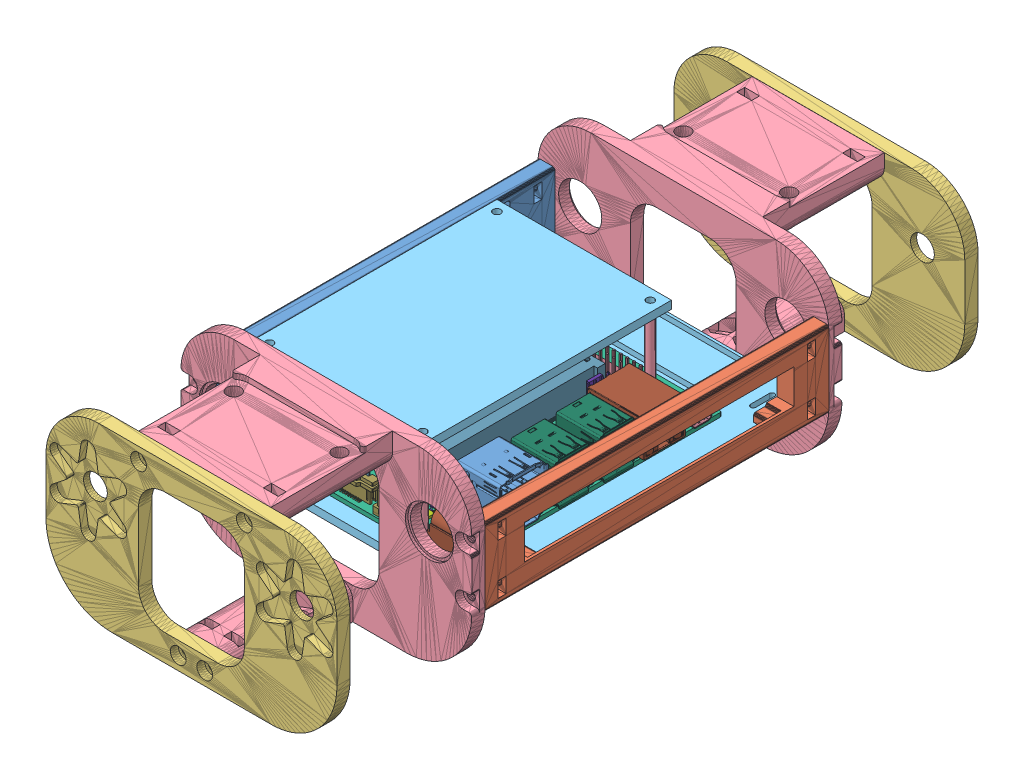
SolidWorks assembly torsol_with_jestson, configuration Default. Lengths in mm. (continued)
Components (placement in the parent): (continued)
- plate_with_jetson-1: plate_with_jetson [Default] at (-139.2728 38.0458 18.6623) x (-1 0 0) z (0 -1 0) size (107 134 44.9) (continued)
  - Jetson nano_fixed.step-1: Jetson nano_fixed.step [Default] at (-69.1681 -61.3023 -1.45) x (0 1 0) z (0 0 -1) size (100 81.03 30.51) (continued)
    - 142-13449-1000-A02_ASM.step-1: 142-13449-1000-A02_ASM.step [Default] at origin size (100 81.03 23.19) (continued)
      - 074-0102-000_4.step-1: 074-0102-000_4.step [Default] at (0.254 44.36 1.575) x (0 1 0) z (0 0 1) size (10.16 5.08 11.6)
      - 064-0400-000_1.step-1: 064-0400-000_1.step [Default] at (73.75 7.77 1.575) size (10.16 5.8 13.5)
      - MEC_STANDOFF_PTH_620C380P.step-1: MEC_STANDOFF_PTH_620C380P.step [Default] at (40.276 40.3 1.575) x (0 1 0) z (0 0 1) size (6.2 6.2 0.73)
      - 090-0231-000_1.step-1: 090-0231-000_1.step [Default] at (35.3 0.7 1.575) x (-1 0 0) z (0 0 1) size (2.5 1.55 0.55)
      - 090-0231-000_1.step-2: 090-0231-000_1.step [Default] at (52.25 0.7 1.575) x (-1 0 0) z (0 0 1) size (2.5 1.55 0.55)
      - 090-0231-000_1.step-3: 090-0231-000_1.step [Default] at (56.05 0.7 1.575) size (2.5 1.55 0.55)
      - 090-0231-000_1.step-4: 090-0231-000_1.step [Default] at (59.65 0.7 1.575) size (2.5 1.55 0.55)
      - 090-0231-000_1.step-5: 090-0231-000_1.step [Default] at (39.1 0.7 1.575) size (2.5 1.55 0.55)
      - 090-0231-000_1.step-6: 090-0231-000_1.step [Default] at (43.1 0.7 1.575) size (2.5 1.55 0.55)
      - 090-0231-000_1.step-7: 090-0231-000_1.step [Default] at (14.6 1.8 1.575) size (2.5 1.55 0.55)
      - 090-0231-000_1.step-8: 090-0231-000_1.step [Default] at (19.1 1.8 1.575) size (2.5 1.55 0.55)
      - 090-0231-000_1.step-9: 090-0231-000_1.step [Default] at (22.5 1.4 1.575) size (2.5 1.55 0.55)
      - 090-0231-000_1.step-10: 090-0231-000_1.step [Default] at (28.45 3.35 1.575) size (2.5 1.55 0.55)
      - 090-0231-000_1.step-11: 090-0231-000_1.step [Default] at (31.65 3.35 1.575) size (2.5 1.55 0.55)
      - 074-0223-000_2.step-1: 074-0223-000_2.step [Default] at (5.85 53.25 1.575) x (0 1 0) z (0 0 1) size (15.24 2.54 11.6)
      - 131-0832-000_2.step-1: 131-0832-000_2.step [Default] at (56.3 54.7 1.575) x (0 -1 0) z (0 0 1) size (4.96 4.06 1.8)
      - 115-0836-000_1.step-1: 115-0836-000_1.step [Default] at (21.1 56.6 1.575) size (2.9 3.58 1.45)
      - 115-0836-000_1.step-2: 115-0836-000_1.step [Default] at (11.8 42.3 1.575) size (2.9 3.58 1.45)
      - 315-0620-000_1.step-1: 315-0620-000_1.step [Default] at (72.1 53.4 1.575) x (0 -1 0) z (0 0 1) size (2.9 3.58 1.1)
      - 315-1062-000_1.step-1: 315-1062-000_1.step [Default] at (26.8 25.15 1.575) x (0 -1 0) z (0 0 1) size (2.9 3.58 1.45)
      - 170-0285-000_1.step-1: 170-0285-000_1.step [Default] at (28.72 57.28 1.575) x (0 1 0) z (0 0 1) size (4.9 7.21 1.75)
      - 115-0138-000_1.step-1: 115-0138-000_1.step [Default] at (9.15 48.55 1.575) x (0 1 0) z (0 0 1) size (2 2.88 1.1)
      - 115-1821-000_1.step-1: 115-1821-000_1.step [Default] at (3.3 40.8 1.575) x (-1 0 0) z (0 0 1) size (2 2.88 1.1)
      - 115-1821-000_1.step-2: 115-1821-000_1.step [Default] at (6.25 39.55 1.575) x (0 -1 0) z (0 0 1) size (2 2.88 1.1)
      - 115-0742-000_2.step-1: 115-0742-000_2.step [Default] at (3.05 46.85 1.575) size (2 2.88 1.1)
      - 115-0742-000_2.step-2: 115-0742-000_2.step [Default] at (3.05 51.65 1.575) x (-1 0 0) z (0 0 1) size (2 2.88 1.1)
      - 115-1821-000_1.step-3: 115-1821-000_1.step [Default] at (59.6 27.6 1.575) x (0 1 0) z (0 0 1) size (2 2.88 1.1)
      - 091-0022-000_1.step-1: 091-0022-000_1.step [Default] at (-0.95 5.7 1.575) size (2 2.51 1.1)
      - 091-0023-000_1.step-1: 091-0023-000_1.step [Default] at (15.25 29.9 1.575) x (0 -1 0) z (0 0 1) size (2 2.51 1.1)
      - 080-1368-000_1.step-1: 080-1368-000_1.step [Default] at (88 -14.3 1.575) size (10.99 7.28 4.95)
      - 080-1656-000_3.step-1: 080-1656-000_3.step [Default] at (44 16.6 1.575) x (-1 0 0) z (0 0 1) size (77.5 25.85 9.76)
      - 090-0243-000_1.step-1: 090-0243-000_1.step [Default] at (8.5 -4.1 1.575) x (-1 0 0) z (0 0 1) size (1.41 0.61 0.45)
      - 090-0243-000_1.step-2: 090-0243-000_1.step [Default] at (9.95 -3.7 1.575) x (0 1 0) z (0 0 1) size (1.41 0.61 0.45)
      - 090-0243-000_1.step-3: 090-0243-000_1.step [Default] at (9.5 -10.95 1.575) x (-1 0 0) z (0 0 1) size (1.41 0.61 0.45)
      - 090-0243-000_1.step-4: 090-0243-000_1.step [Default] at (9.8 -6.25 1.575) x (-1 0 0) z (0 0 1) size (1.41 0.61 0.45)
      - 090-0243-000_1.step-5: 090-0243-000_1.step [Default] at (9.5 -9.5 1.575) x (-1 0 0) z (0 0 1) size (1.41 0.61 0.45)
      - 090-0172-000_1.step-1: 090-0172-000_1.step [Default] at (90.6 -5 1.575) size (1.41 0.61 0.55)
      - 090-0172-000_1.step-2: 090-0172-000_1.step [Default] at (88.8 -5 1.575) x (-1 0 0) z (0 0 1) size (1.41 0.61 0.55)
      - 115-2177-000_2.step-1: 115-2177-000_2.step [Default] at (12.7 51.35 1.575) x (0 1 0) z (0 0 1) size (1.8 1.71 0.4)
      - 090-0233-000_1.step-1: 090-0233-000_1.step [Default] at (83.5 -6.6 1.575) size (3.3 1.3 0.74)
      - 064-0374-000_2.step-1: 064-0374-000_2.step [Default] at (19.75 -9.65 1.575) size (18.11 18.56 21.86)
      - 115-2628-000_3.step-1: 115-2628-000_3.step [Default] at (25.2 41.2 1.575) size (9.5 9.5 0.9)
      - 092-0073-000_1.step-1: 092-0073-000_1.step [Default] at (93.35 -4.75 1.575) x (-1 0 0) z (0 0 1) size (2.46 0.81 0.9)
      - IND_SMD_0402_H060.step-1: IND_SMD_0402_H060.step [Default] at (12.85 29.9 1.575) x (-1 0 0) z (0 0 1) size (1 0.5 0.6)
      - 1206_H190.step-1: 1206_H190.step [Default] at (82 18.8 1.575) x (0 1 0) z (0 0 1) size (3.2 1.6 1.9)
      - 1206_H190.step-2: 1206_H190.step [Default] at (81.95 13.5 1.575) x (0 -1 0) z (0 0 1) size (3.2 1.6 1.9)
      - 300-0868-000_3.step-1: 300-0868-000_3.step [Default] at (69.6 4 1.575) x (-1 0 0) z (0 0 1) size (1 0.6 0.4)
      - 300-0868-000_3.step-2: 300-0868-000_3.step [Default] at (9.55 0.95 1.575) size (1 0.6 0.4)
      - 300-0868-000_3.step-3: 300-0868-000_3.step [Default] at (19.6 31.45 1.575) x (0 -1 0) z (0 0 1) size (1 0.6 0.4)
      - 300-0868-000_3.step-4: 300-0868-000_3.step [Default] at (91.45 -2.45 1.575) x (-1 0 0) z (0 0 1) size (1 0.6 0.4)
      - 300-0868-000_3.step-5: 300-0868-000_3.step [Default] at (84.6 -5.1 1.575) size (1 0.6 0.4)
      - 300-0868-000_3.step-6: 300-0868-000_3.step [Default] at (66.725 5.875 1.575) x (0 -1 0) z (0 0 1) size (1 0.6 0.4)
      - 300-0868-000_3.step-7: 300-0868-000_3.step [Default] at (20.8 31.45 1.575) x (0 -1 0) z (0 0 1) size (1 0.6 0.4)
      - 300-0868-000_3.step-8: 300-0868-000_3.step [Default] at (62.9 31.35 1.575) x (-1 0 0) z (0 0 1) size (1 0.6 0.4)
      - 300-0868-000_3.step-9: 300-0868-000_3.step [Default] at (65.475 4.8 1.575) x (-1 0 0) z (0 0 1) size (1 0.6 0.4)
      - 300-0868-000_3.step-10: 300-0868-000_3.step [Default] at (63.9 33.85 1.575) x (-1 0 0) z (0 0 1) size (1 0.6 0.4)
      - 300-0868-000_3.step-11: 300-0868-000_3.step [Default] at (15.65 27.9 1.575) size (1 0.6 0.4)
      - 300-0868-000_3.step-12: 300-0868-000_3.step [Default] at (11.8 6.1 1.575) x (0 1 0) z (0 0 1) size (1 0.6 0.4)
      - 300-0868-000_3.step-13: 300-0868-000_3.step [Default] at (22.1 6.25 1.575) x (0 1 0) z (0 0 1) size (1 0.6 0.4)
      - 300-0869-000_3.step-1: 300-0869-000_3.step [Default] at (9.65 8.1 1.575) x (0 -1 0) z (0 0 1) size (1 0.6 0.53)
      - 300-0402-000_1.step-1: 300-0402-000_1.step [Default] at (20.8 26.45 1.575) x (0 -1 0) z (0 0 1) size (2 2.69 1.1)
      - 300-0560-000_1.step-1: 300-0560-000_1.step [Default] at (6.8 43.65 1.575) x (-1 0 0) z (0 0 1) size (2 2.69 1.1)
      - 174-0159-000_2.step-1: 174-0159-000_2.step [Default] at (61.49 57.15 1.575) x (-1 0 0) z (0 0 1) size (2 3.52 0.6)
      - 064-0373-000_2.step-1: 064-0373-000_2.step [Default] at (72.95 -7.825 1.575) size (17.8 21.61 17.46)
      - 064-0375-000_2.step-1: 064-0375-000_2.step [Default] at (19.751 -12.275 1.575) size (16.2 5.58 0.01)
      - 074-0221-000_3.step-1: 074-0221-000_3.step [Default] at (86 29 1.575) x (0 1 0) z (0 0 1) size (50.8 5.08 11.6)
      - 2016MM_H100.step-1: 2016MM_H100.step [Default] at (24.5 49.25 1.575) x (0 1 0) z (0 0 1) size (2 1.6 1)
      - 065-0656-000_2.step-1: 065-0656-000_2.step [Default] at (55.6 -10.04 1.575) x (-1 0 0) z (0 0 1) size (16.19 17.45 19.62)
      - 065-0656-000_2.step-2: 065-0656-000_2.step [Default] at (38.6 -10.04 1.575) x (-1 0 0) z (0 0 1) size (16.19 17.45 19.62)
      - 115-1921-000_3.step-1: 115-1921-000_3.step [Default] at (80.45 50.52 1.575) x (0 -1 0) z (0 0 1) size (5 4 1)
      - 115-1921-000_3.step-2: 115-1921-000_3.step [Default] at (80.4 34.5 1.575) x (0 -1 0) z (0 0 1) size (5 4 1)
      - 115-1921-000_3.step-3: 115-1921-000_3.step [Default] at (77.2 25.9 1.575) x (0 -1 0) z (0 0 1) size (5 4 1)
      - 085-0328-000_2.step-1: 085-0328-000_2.step [Default] at (16.28 36.32 1.575) x (0 -1 0) z (0 0 1) size (3.81 2.5 0.6)
      - 074-0216-000_2.step-1: 074-0216-000_2.step [Default] at (92.14 58 1.575) x (-1 0 0) z (0 0 1) size (4.83 5 11.5)
      - 060-0002-000_1.step-1: 060-0002-000_1.step [Default] at (41.2 57.9 1.575) x (0 -1 0) z (0 0 1) size (5.1 5.4 1.68)
      - 316-0697-000_1.step-1: 316-0697-000_1.step [Default] at (50.6 58.1 1.575) x (0 -1 0) z (0 0 1) size (3 3.72 0.8)
      - 032-0256-000_1.step-1: 032-0256-000_1.step [Default] at (5.925 9.425 1.575) size (4.22 2.82 2)
      - 041-0092-000_1.step-1: 041-0092-000_1.step [Default] at (46.9 54.9 1.575) x (0 -1 0) z (0 0 1) size (4.22 2.82 1.2)
      - 080-1243-000_3.step-1: 080-1243-000_3.step [Default] at (69.9 40.3 1.575) x (0 -1 0) z (0 0 1) size (21.9 9.1 4.8)
      - 102-0066-000_2.step-1: 102-0066-000_2.step [Default] at (18 4.2 1.575) size (1 1.86 0.61)
      - 102-0066-000_2.step-2: 102-0066-000_2.step [Default] at (13.55 4.2 1.575) size (1 1.86 0.61)
      - 102-0066-000_2.step-3: 102-0066-000_2.step [Default] at (32.45 5.81 1.575) size (1 1.86 0.61)
      - 102-0066-000_2.step-4: 102-0066-000_2.step [Default] at (27.65 5.81 1.575) size (1 1.86 0.61)
      - 102-0066-000_2.step-5: 102-0066-000_2.step [Default] at (20.15 4.2 1.575) size (1 1.86 0.61)
      - 102-0066-000_2.step-6: 102-0066-000_2.step [Default] at (15.75 4.2 1.575) size (1 1.86 0.61)
      - 102-0066-000_2.step-7: 102-0066-000_2.step [Default] at (29.25 5.81 1.575) size (1 1.86 0.61)
      - 102-0066-000_2.step-8: 102-0066-000_2.step [Default] at (30.85 5.81 1.575) size (1 1.86 0.61)
      - 102-0037-000_1.step-1: 102-0037-000_1.step [Default] at (55.2 2.95 1.575) x (-1 0 0) z (0 0 1) size (1 1.86 0.91)
      - 102-0037-000_1.step-2: 102-0037-000_1.step [Default] at (39.99 2.87 1.575) x (-1 0 0) z (0 0 1) size (1 1.86 0.91)
      - 102-0037-000_1.step-3: 102-0037-000_1.step [Default] at (60.55 2.95 1.575) x (-1 0 0) z (0 0 1) size (1 1.86 0.91)
      - 102-0037-000_1.step-4: 102-0037-000_1.step [Default] at (38.22 2.87 1.575) x (-1 0 0) z (0 0 1) size (1 1.86 0.91)
      - 0805_H140.step-1: 0805_H140.step [Default] at (8.1 -2.1 1.575) size (2.01 1.25 1.4)
      - 0805_H150.step-1: 0805_H150.step [Default] at (82.9 -8.4 1.575) x (-1 0 0) z (0 0 1) size (2.01 1.25 1.5)
      - 0603_H100.step-1: 0603_H100.step [Default] at (6.1 41.525 1.575) x (-1 0 0) z (0 0 1) size (1.6 0.81 1)
      - 0603_H060.step-1: 0603_H060.step [Default] at (63.25 -12 1.575) x (0 1 0) z (0 0 1) size (1.6 0.81 0.6)
      - 0603_H060.step-2: 0603_H060.step [Default] at (63.8 -0.7 1.575) x (0 -1 0) z (0 0 1) size (1.6 0.81 0.6)
      - 0603_H060.step-3: 0603_H060.step [Default] at (82.4 -10 1.575) x (-1 0 0) z (0 0 1) size (1.6 0.81 0.6)
      - 0603_H100.step-2: 0603_H100.step [Default] at (9.486 -7.5 1.575) x (-1 0 0) z (0 0 1) size (1.6 0.81 1)
      - 0603_H100.step-3: 0603_H100.step [Default] at (17.4 57.4 1.575) x (0 -1 0) z (0 0 1) size (1.6 0.81 1)
      - 0603_H100.step-4: 0603_H100.step [Default] at (30.35 25.9 1.575) x (0 -1 0) z (0 0 1) size (1.6 0.81 1)
      - 0603_H100.step-5: 0603_H100.step [Default] at (11.4 45.7 1.575) size (1.6 0.81 1)
      - 0603_H100.step-6: 0603_H100.step [Default] at (3.2 43 1.575) size (1.6 0.81 1)
      - 0603_H100.step-7: 0603_H100.step [Default] at (74.7 53.4 1.575) x (0 -1 0) z (0 0 1) size (1.6 0.81 1)
      - 0603_H100.step-8: 0603_H100.step [Default] at (69.5 53.9 1.575) x (0 -1 0) z (0 0 1) size (1.6 0.81 1)
      - 0603_H100.step-9: 0603_H100.step [Default] at (52.5 52.9 1.575) x (-1 0 0) z (0 0 1) size (1.6 0.81 1)
      - 0603_H100.step-10: 0603_H100.step [Default] at (52.5 54.2 1.575) x (-1 0 0) z (0 0 1) size (1.6 0.81 1)
      - 0603_H100.step-11: 0603_H100.step [Default] at (27.3 51.35 1.575) size (1.6 0.81 1)
      - 0603_H100.step-12: 0603_H100.step [Default] at (22.7 49.1 1.575) x (0 1 0) z (0 0 1) size (1.6 0.81 1)
      - 0603_H100.step-13: 0603_H100.step [Default] at (26.2 48.8 1.575) x (0 1 0) z (0 0 1) size (1.6 0.81 1)
      - 0603_H100.step-14: 0603_H100.step [Default] at (20.9 49.1 1.575) x (0 1 0) z (0 0 1) size (1.6 0.81 1)
      - 0603_H100.step-15: 0603_H100.step [Default] at (65.5 27.4 1.575) x (0 -1 0) z (0 0 1) size (1.6 0.81 1)
      - 0603_H100.step-16: 0603_H100.step [Default] at (63.8 52.2 1.575) x (-1 0 0) z (0 0 1) size (1.6 0.81 1)
      - 0603_H100.step-17: 0603_H100.step [Default] at (52.5 55.4 1.575) x (-1 0 0) z (0 0 1) size (1.6 0.81 1)
      - 080-1669-000_2.step-1: 080-1669-000_2.step [Default] at (0.2 29 1.575) x (0 -1 0) z (0 0 1) size (22.4 5.4 7.7)
    - 244-63448-0000-000_ASM.step-1: 244-63448-0000-000_ASM.step [Default] at (11.2 22.5 8.2712) size (69.6 45 21.37)
      - 142-13448-1000-A02_ASM.step-1: 142-13448-1000-A02_ASM.step [Default] at origin size (23 37.01 4.01)
        - 080-0051-000_3.step-1: 080-0051-000_3.step [Default] at (28.331 29.139 0) x (-1 0 0) z (0 0 -1) size (13.4 17 1.28)
        - TM670M-A2_1.step-1: TM670M-A2_1.step [Default] at (23.7 13.45 1.2) size (23 23 1.29)
      - 142-13448-1000-A02-SKU0000_ASM.step-1: 142-13448-1000-A02-SKU0000_ASM.step [Default] at origin size (23 23 1.29)
        - TM670M-A2_1.step-1: TM670M-A2_1.step [Default] at (23.7 13.45 1.2) size (23 23 1.29)
      - PORG_HSK_ASSY_ASM.step-1: PORG_HSK_ASSY_ASM.step [Default] at (0 0 4.01) size (58.7 39.4 17.3)
        - PORG_HEAT_SINK.step-1: PORG_HEAT_SINK.step [Default] at origin size (58.7 39.4 17.3)
      - 142-63448-1GEN_A00.step-1: 142-63448-1GEN_A00.step [Default] at origin size (69.6 45 1.2)
      - PORG_LEAF_SPRING_DRAWN.step-1: PORG_LEAF_SPRING_DRAWN.step [Default] at (0 0 -0.4) x (1 0.000001 0) z (0 0 1) size (39.83 21.3 1.2)
      - PORG_LEAF_SPRING_SCREW.step-1: PORG_LEAF_SPRING_SCREW.step [Default] at (6.9871 5.9982 5.21) x (0 0 -1) z (0 1 0) size (6.41 4.7 4.7)
      - PORG_LEAF_SPRING_SCREW.step-2: PORG_LEAF_SPRING_SCREW.step [Default] at (6.9871 20.9018 5.21) x (0 0 -1) z (0 1 0) size (6.41 4.7 4.7)
      - PORG_LEAF_SPRING_SCREW.step-3: PORG_LEAF_SPRING_SCREW.step [Default] at (40.4129 20.9018 5.21) x (0 0 -1) z (0 1 0) size (6.41 4.7 4.7)
      - PORG_LEAF_SPRING_SCREW.step-4: PORG_LEAF_SPRING_SCREW.step [Default] at (40.4129 5.9982 5.21) x (0 0 -1) z (0 1 0) size (6.41 4.7 4.7)
    - PORG_HEX_STANDOFF.step-1: PORG_HEX_STANDOFF.step [Default] at (75.8 58.5 8.17) x (-1 0 0) z (0 0 -1) size (5.14 4.45 6.57)
    - PORG_HEX_STANDOFF.step-2: PORG_HEX_STANDOFF.step [Default] at (12.2 58.5 8.17) x (-1 0 0) z (0 0 -1) size (5.14 4.45 6.57)
    - PORG_SYSTEM_SCREW.step-1: PORG_SYSTEM_SCREW.step [Default] at (12.2 58.5 3.73) size (4.55 4.55 4.53)
    - PORG_SYSTEM_SCREW.step-2: PORG_SYSTEM_SCREW.step [Default] at (75.8 58.5 3.73) size (4.55 4.55 4.53)
    - PORG_SYSTEM_SCREW.step-3: PORG_SYSTEM_SCREW.step [Default] at (75.8 58.5 5.67) x (-1 0 0) z (0 0 -1) size (4.55 4.55 4.53)
    - PORG_SYSTEM_SCREW.step-4: PORG_SYSTEM_SCREW.step [Default] at (12.2 58.5 5.67) x (-1 0 0) z (0 0 -1) size (4.55 4.55 4.53)
    - 155-0576-000.step-1: 155-0576-000.step [Default] at (40.276 40.3 5.01) size (5 5 4)
  - battery_4000mah_2s-1: battery_4000mah_2s [Default] at (-88.6681 62.6977 -1.45) x (1 0 0) z (0 -1 0) size (85 42 27) (hidden)
- copper_cylinder_jetson-1: copper_cylinder_jetson [Default] at (-70.1047 41.0708 -6.0354) x (-0.061328 0 0.998118) z (0 1 0) size (3 3 30)
- copper_cylinder_jetson-5: copper_cylinder_jetson [Default] at (-128.1047 71.0708 -6.0354) x (0.951181 0 0.308634) z (0 -1 0) size (3 3 30)
- copper_cylinder_jetson-6: copper_cylinder_jetson [Default] at (-128.1047 71.0708 79.9646) x (0.479614 0 0.877479) z (0 -1 0) size (3 3 30)
- copper_cylinder_jetson-7: copper_cylinder_jetson [Default] at (-70.1047 71.0708 79.9646) x (-0.839782 0 0.542924) z (0 -1 0) size (3 3 30)
- plate_top_jetson-1: plate_top_jetson [Default] at (-99.1047 74.0708 38.2298) x (-1 0 0) z (0 -1 0) size (66 94 3)
Mates (geometry in assembly coordinates):
- Coincident9: coincident anti-aligned: plane of non-mega_L_side_plate-2 through (-41.8547 39.5958 -42.0354) normal (0 0 -1); plane of I_shoulder_mg-1 through (-38.6047 81.5958 -42.0354) normal (0 0 1)
- Parallel3: parallel anti-aligned: plane of R_side_plate-1 through (-145.3547 -0.5404 -42.0354) normal (0 0 -1); plane of I_shoulder_mg-1 through (-38.6047 81.5958 -42.0354) normal (0 0 1)
- Parallel5: parallel aligned: plane of R_side_plate-1 through (-145.3547 63.4596 -42.0354) normal (0 1 0); plane of I_shoulder_mg-1 through (-38.6047 81.5958 -42.0354) normal (0 1 0)
- Coincident20: coincident aligned: plane of R_side_plate-1 through (-148.6047 -0.5404 -42.0354) normal (-1 0 0); plane of I_shoulder_mg-1 through (-148.6047 81.5958 -42.0354) normal (-1 0 0)
- Coincident22: coincident: point of R_side_plate-1; plane of I_shoulder_mg-1 through (-66.0912 117.4171 -42.0354) normal (-0.60876 0.793355 0)
- Coincident23: coincident anti-aligned: plane of non-mega_L_side_plate-2 through (-41.8547 39.5958 87.9646) normal (0 0 1); plane of I_shoulder_mg-2 through (-148.6047 81.4596 87.9646) normal (0 0 -1)
- Coincident24: coincident aligned: plane of R_side_plate-1 through (-148.6047 -0.5404 -42.0354) normal (-1 0 0); plane of I_shoulder_mg-2 through (-148.6047 81.4596 87.9646) normal (-1 0 0)
- Parallel7: parallel aligned: plane of R_side_plate-1 through (-145.3547 63.4596 -42.0354) normal (0 1 0); plane of I_shoulder_mg-2 through (-148.6047 81.4596 87.9646) normal (0 1 0)
- Coincident26: coincident: plane of R_side_plate-1 through (-137.9269 55.8817 -42.0354) normal (0.13052 0.991446 0); point of I_shoulder_mg-2
- Coincident27: coincident anti-aligned: plane of O_shoulder-1 through (-38.1905 81.6503 -93.0354) normal (0 0 1); plane of I_shoulder_mg-1 through (-38.6047 81.5958 -93.0354) normal (0 0 -1)
- Parallel8: parallel anti-aligned: plane of O_shoulder-1 through (-38.1905 13.6503 -93.0354) normal (0 -1 0); plane of I_shoulder_mg-1 through (-38.6047 79.5958 -42.0354) normal (0 1 0)
- Coincident29: coincident: point of O_shoulder-1; point of I_shoulder_mg-1
- Coincident30: coincident anti-aligned: plane of O_shoulder-2 through (-148.6047 81.4596 138.9646) normal (0 0 -1); plane of I_shoulder_mg-2 through (-148.6047 81.4596 138.9646) normal (0 0 1)
- Parallel9: parallel anti-aligned: plane of I_shoulder_mg-2 through (-148.6047 79.4596 87.9646) normal (0 1 0); plane of O_shoulder-2 through (-148.6047 13.4596 138.9646) normal (0 -1 0)
- Coincident32: coincident: point of I_shoulder_mg-2; point of O_shoulder-2
- Coincident33: coincident anti-aligned: plane of R_side_plate-1 through (-145.3547 -0.5404 87.9646) normal (0 0 1); plane of I_shoulder_mg-2 through (-148.6047 81.4596 87.9646) normal (0 0 -1)
- Coincident34: coincident: point of non-mega_L_side_plate-2; point of I_shoulder_mg-1
- Parallel10: parallel aligned: plane of non-mega_L_side_plate-2 through (-41.8547 63.5958 -42.0354) normal (0 1 0); plane of I_shoulder_mg-1 through (-38.6047 81.5958 -42.0354) normal (0 1 0)
- Coincident35: coincident anti-aligned: plane of non-mega_L_side_plate-2 through (-41.8547 36.5958 -42.0354) normal (0 1 0); plane of plate_with_jetson-1/plate_jetson-1 through (-93.1047 36.5958 22.4646) normal (0 -1 0)
- Coincident36: coincident anti-aligned: plane of non-mega_L_side_plate-2 through (-39.6047 39.5958 -42.0354) normal (-1 0 0); plane of plate_with_jetson-1/plate_jetson-1 through (-39.6047 36.5958 69.9646) normal (1 0 0)
- Distance1: distance = 1 mm anti-aligned: plane of plate_with_jetson-1/plate_jetson-1 through (-39.6047 36.5958 69.9646) normal (0 0 1); plane of non-mega_L_side_plate-2 through (-41.8547 39.5958 70.9646) normal (0 0 -1)
- Concentric1: concentric anti-aligned: circle of plate_with_jetson-1/Jetson nano_fixed.step-1/142-13449-1000-A02_ASM.step-1/142-13449-1000-A02.step-1; cylinder of copper_cylinder_jetson-1 through (-70.1047 71.0708 -6.0354) axis (0 -1 0) radius 1.5
- Coincident38: coincident anti-aligned: plane of plate_with_jetson-1/Jetson nano_fixed.step-1/142-13449-1000-A02_ASM.step-1/142-13449-1000-A02.step-1 through (-70.1047 41.0708 79.9646) normal (0 1 0); plane of copper_cylinder_jetson-1 through (-70.1047 41.0708 -6.0354) normal (0 -1 0)
- Concentric2: concentric anti-aligned: circle of plate_with_jetson-1/Jetson nano_fixed.step-1/142-13449-1000-A02_ASM.step-1/142-13449-1000-A02.step-1; circle of copper_cylinder_jetson-5
- Coincident39: coincident anti-aligned: plane of plate_with_jetson-1/Jetson nano_fixed.step-1/142-13449-1000-A02_ASM.step-1/142-13449-1000-A02.step-1 through (-70.1047 41.0708 79.9646) normal (0 1 0); plane of copper_cylinder_jetson-5 through (-128.1047 41.0708 -6.0354) normal (0 -1 0)
- Concentric3: concentric anti-aligned: circle of plate_with_jetson-1/Jetson nano_fixed.step-1/142-13449-1000-A02_ASM.step-1/142-13449-1000-A02.step-1; circle of copper_cylinder_jetson-6
- Coincident40: coincident anti-aligned: plane of plate_with_jetson-1/Jetson nano_fixed.step-1/142-13449-1000-A02_ASM.step-1/142-13449-1000-A02.step-1 through (-70.1047 41.0708 79.9646) normal (0 1 0); plane of copper_cylinder_jetson-6 through (-128.1047 41.0708 79.9646) normal (0 -1 0)
- Concentric4: concentric anti-aligned: circle of plate_with_jetson-1/Jetson nano_fixed.step-1/142-13449-1000-A02_ASM.step-1/142-13449-1000-A02.step-1; circle of copper_cylinder_jetson-7
- Coincident43: coincident anti-aligned: plane of plate_with_jetson-1/Jetson nano_fixed.step-1/142-13449-1000-A02_ASM.step-1/142-13449-1000-A02.step-1 through (-70.1047 41.0708 79.9646) normal (0 1 0); plane of copper_cylinder_jetson-7 through (-70.1047 41.0708 79.9646) normal (0 -1 0)
- Coincident45: coincident anti-aligned: plane of copper_cylinder_jetson-6 through (-128.1047 71.0708 79.9646) normal (0 1 0); plane of plate_top_jetson-1 through (-99.1047 71.0708 38.2298) normal (0 -1 0)
- Concentric8: concentric aligned: circle of copper_cylinder_jetson-6; circle of plate_top_jetson-1
- Concentric9: concentric anti-aligned: circle of copper_cylinder_jetson-1; circle of plate_top_jetson-1
